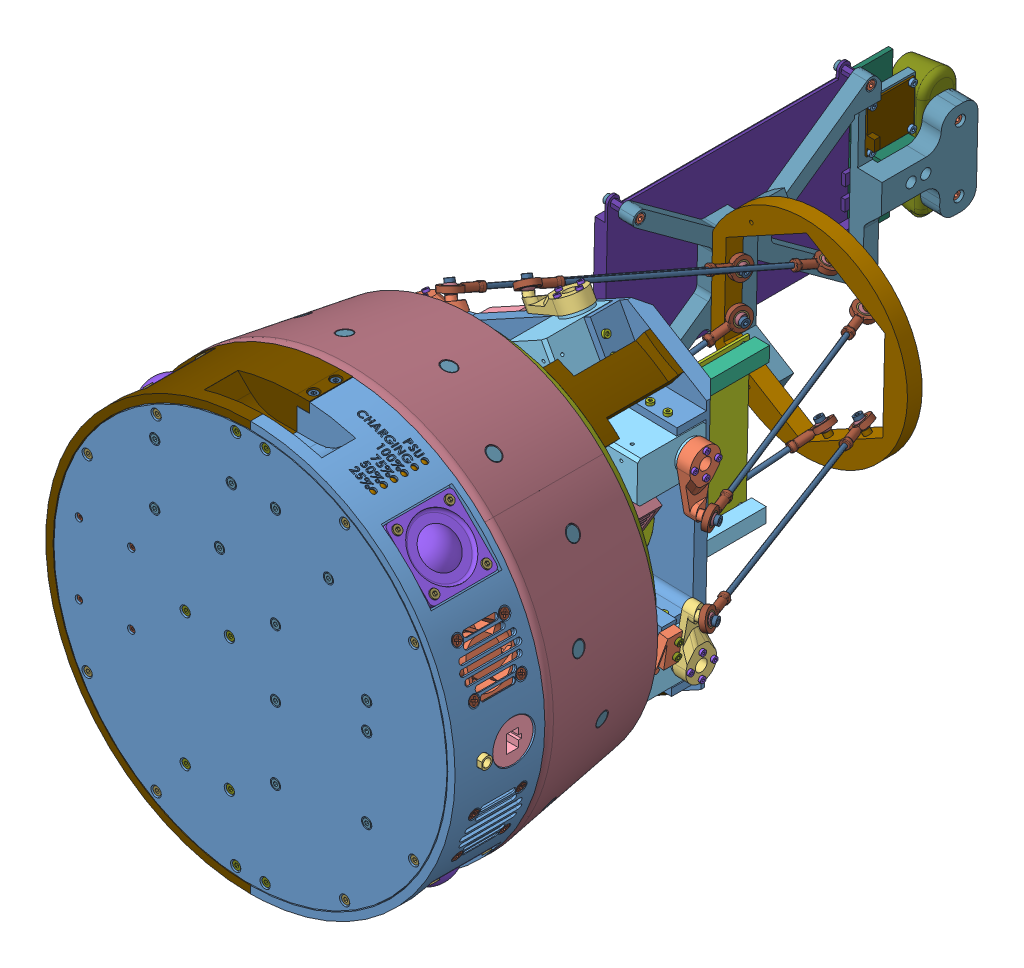
SolidWorks assembly robot, configuration Défaut. Lengths in mm. (continued)
Components (placement in the parent): (continued)
- stewart-1: stewart [Défaut] at (-73.8927 -28.7791 -12.2571) x (-0.023118 -0.999733 0) z (0 0 1) size (242.48 224.83 213.52)
  - stewart bottom-1: stewart bottom [Défaut] at (6.7039 12.5905 32.3281) size (242.48 216.75 132.5)
    - stewart bottom-1: stewart bottom [Défaut] at (-52.7025 18.5554 219.9038) size (234.9 203.43 30)
    - XL430-W250-T-1: XL430-W250-T [Défaut] at (-127.7192 44.5266 253.1538) x (-0.5 0.866025 0) z (-0.866025 -0.5 0) size (28.5 46.5 36)
    - XL430-W250-T-2: XL430-W250-T [Défaut] at (-112.7025 70.5362 253.1538) x (1 0 0) z (0 1 0) size (28.5 46.5 36)
    - XL430-W250-T-3: XL430-W250-T [Défaut] at (7.2975 70.5362 253.1538) x (1 0 0) z (0 1 0) size (28.5 46.5 36)
    - XL430-W250-T-4: XL430-W250-T [Défaut] at (22.3142 44.5266 253.1538) x (-0.5 -0.866025 0) z (0.866025 -0.5 0) size (28.5 46.5 36)
    - XL430-W250-T-5: XL430-W250-T [Défaut] at (-37.6858 -59.3965 253.1538) x (-0.5 -0.866025 0) z (0.866025 -0.5 0) size (28.5 46.5 36)
    - XL430-W250-T-6: XL430-W250-T [Défaut] at (-67.7192 -59.3965 253.1538) x (-0.5 0.866025 0) z (-0.866025 -0.5 0) size (28.5 46.5 36)
    - stewart horn (left)-1: stewart horn (left) [Défaut] at (-112.7025 116.5362 241.1538) x (1 0 0) z (0 -1 0) size (45.5 21 11.31)
    - stewart horn (right)-1: stewart horn (right) [Défaut] at (7.2975 116.5362 241.1538) x (-1 0 0) z (0 -1 0) size (45.5 21 11.31)
    - USB hub support-1: USB hub support [Défaut] at (-103.8877 -42.7506 219.9038) x (-0.866025 -0.5 0) z (0.5 -0.866025 0) size (24.57 17.21 30)
    - USB hub support-2: USB hub support [Défaut] at (-136.8877 14.407 219.9038) x (-0.866025 -0.5 0) z (0.5 -0.866025 0) size (24.57 17.21 30)
    - USB hub support-3: USB hub support [Défaut] at (-16.5172 -68.7314 219.9038) x (0.866025 -0.5 0) z (0.5 0.866025 0) size (24.57 17.21 30)
    - USB hub support-4: USB hub support [Défaut] at (16.4828 -11.5737 219.9038) x (0.866025 -0.5 0) z (0.5 0.866025 0) size (24.57 17.21 30)
    - OpenCR support 1-1: OpenCR support 1 [Défaut] at (-9.7025 62.0362 219.9038) x (-1 0 0) z (0 -1 0) size (20 76 23)
    - OpenCR support 2-1: OpenCR support 2 [Défaut] at (-95.7025 62.0362 219.9038) x (-1 0 0) z (0 -1 0) size (20 76 23)
    - OpenCR-1: OpenCR [Défaut] at (-52.7025 47.4362 181.9038) x (1 0 0) z (0 1 0) size (110.25 75 17.6)
    - Anker USB-c hub (4 ports)-1: Anker USB-c hub (4 ports) [Défaut] at (3.7083 -8.7432 211.4339) x (-0.5 -0.866025 0) z (-0.496732 0.286788 -0.819152) size (96 30 21)
    - Anker USB-c hub (4 ports)-2: Anker USB-c hub (4 ports) [Défaut] at (-109.4441 -8.9342 211.1664) x (0.5 -0.866025 0) z (0.496732 0.286788 -0.819152) size (96 30 21)
    - M2.5x8mm plastic-1: M2.5x8mm plastic [Défaut] at (-0.7025 93.5362 232.1538) x (-1 0 0) z (0 0 -1) size (4.5 4.5 9.9)
    - M2.5x8mm plastic-2: M2.5x8mm plastic [Défaut] at (15.2975 93.5362 232.1538) x (-1 0 0) z (0 0 -1) size (4.5 4.5 9.9)
    - M2.5x8mm plastic-3: M2.5x8mm plastic [Défaut] at (46.2328 39.9548 232.1538) x (-1 0 0) z (0 0 -1) size (4.5 4.5 9.9)
    - M2.5x8mm plastic-4: M2.5x8mm plastic [Défaut] at (38.2328 26.0984 232.1538) x (-1 0 0) z (0 0 -1) size (4.5 4.5 9.9)
    - M2.5x8mm plastic-5: M2.5x8mm plastic [Défaut] at (19.2975 93.5362 245.1538) x (0 -0.924225 -0.381849) z (1 0 0) size (4.5 4.5 9.9)
    - M2.5x8mm plastic-6: M2.5x8mm plastic [Défaut] at (19.2975 81.5362 245.1538) x (0 0 1) z (1 0 0) size (4.5 4.5 9.9)
    - M2.5x8mm plastic-7: M2.5x8mm plastic [Défaut] at (37.8404 49.4189 245.1538) x (0.75 -0.433013 -0.5) z (0.5 0.866025 0) size (4.5 4.5 9.9)
    - M2.5x8mm plastic-8: M2.5x8mm plastic [Défaut] at (48.2328 43.4189 245.1538) x (0.75 -0.433013 -0.5) z (0.5 0.866025 0) size (4.5 4.5 9.9)
    - M2.5x8mm plastic-9: M2.5x8mm plastic [Défaut] at (-4.7025 93.5362 245.1538) x (0 0 1) z (-1 0 0) size (4.5 4.5 9.9)
    - M2.5x8mm plastic-10: M2.5x8mm plastic [Défaut] at (-4.7025 81.5362 245.1538) x (0 0 1) z (-1 0 0) size (4.5 4.5 9.9)
    - M2.5x8mm plastic-11: M2.5x8mm plastic [Défaut] at (36.2328 22.6343 245.1538) x (-0.75 0.433013 -0.5) z (-0.5 -0.866025 0) size (4.5 4.5 9.9)
    - M2.5x8mm plastic-12: M2.5x8mm plastic [Défaut] at (25.8404 28.6343 245.1538) x (-0.75 0.433013 -0.5) z (-0.5 -0.866025 0) size (4.5 4.5 9.9)
    - M2x12mm socket-1: M2x12mm socket [Défaut] at (-112.7025 103.5362 233.1538) x (1 0 0) z (0 1 0) size (3.8 3.8 13.6)
    - M2x12mm socket-2: M2x12mm socket [Défaut] at (-104.7025 103.5362 241.1538) x (1 0 0) z (0 1 0) size (3.8 3.8 13.6)
    - M2x12mm socket-3: M2x12mm socket [Défaut] at (-112.7025 103.5362 249.1538) x (1 0 0) z (0 1 0) size (3.8 3.8 13.6)
    - M2x12mm socket-4: M2x12mm socket [Défaut] at (-120.7025 103.5362 241.1538) x (1 0 0) z (0 1 0) size (3.8 3.8 13.6)
    - M2x12mm socket-5: M2x12mm socket [Défaut] at (7.2975 103.5362 233.1538) x (1 0 0) z (0 1 0) size (3.8 3.8 13.6)
    - M2x12mm socket-6: M2x12mm socket [Défaut] at (-0.7025 103.5362 241.1538) x (1 0 0) z (0 1 0) size (3.8 3.8 13.6)
    - M2x12mm socket-7: M2x12mm socket [Défaut] at (7.2975 103.5362 249.1538) x (1 0 0) z (0 1 0) size (3.8 3.8 13.6)
    - M2x12mm socket-8: M2x12mm socket [Défaut] at (15.2975 103.5362 241.1538) x (1 0 0) z (0 1 0) size (3.8 3.8 13.6)
    - M3x12mm plastic-1: M3x12mm plastic [Défaut] at (-126.6425 11.6619 225.9038) x (-0.923728 -0.383049 0) z (0 0 -1) size (5.5 5.5 14.3)
    - M3x12mm plastic-2: M3x12mm plastic [Défaut] at (-119.1425 -1.3285 225.9038) x (-0.923728 -0.383049 0) z (0 0 -1) size (5.5 5.5 14.3)
    - M3x12mm plastic-3: M3x12mm plastic [Défaut] at (-93.6425 -45.4958 225.9038) x (-1 0 0) z (0 0 -1) size (5.5 5.5 14.3)
    - M3x12mm plastic-4: M3x12mm plastic [Défaut] at (-86.1425 -58.4862 225.9038) x (-1 0 0) z (0 0 -1) size (5.5 5.5 14.3)
    - M3x12mm plastic-5: M3x12mm plastic [Défaut] at (-19.2624 -58.4862 225.9038) x (-1 0 0) z (0 0 -1) size (5.5 5.5 14.3)
    - M3x12mm plastic-6: M3x12mm plastic [Défaut] at (-11.7624 -45.4958 225.9038) x (-0.923728 -0.383049 0) z (0 0 -1) size (5.5 5.5 14.3)
    - M3x12mm plastic-7: M3x12mm plastic [Défaut] at (13.7376 -1.3285 225.9038) x (-1 0 0) z (0 0 -1) size (5.5 5.5 14.3)
    - M3x12mm plastic-8: M3x12mm plastic [Défaut] at (21.2376 11.6619 225.9038) x (-1 0 0) z (0 0 -1) size (5.5 5.5 14.3)
    - M3x12mm plastic-9: M3x12mm plastic [Défaut] at (-110.7025 57.0362 225.9038) x (-0.923728 -0.383049 0) z (0 0 -1) size (5.5 5.5 14.3)
    - M3x12mm plastic-10: M3x12mm plastic [Défaut] at (-100.7025 67.0362 225.9038) x (-1 0 0) z (0 0 -1) size (5.5 5.5 14.3)
    - M3x12mm plastic-11: M3x12mm plastic [Défaut] at (-4.7025 67.0362 225.9038) x (-1 0 0) z (0 0 -1) size (5.5 5.5 14.3)
    - M3x12mm plastic-12: M3x12mm plastic [Défaut] at (5.2975 57.0362 225.9038) x (-1 0 0) z (0 0 -1) size (5.5 5.5 14.3)
    - M3x8mm plastic-1: M3x8mm plastic [Défaut] at (-4.7025 55.4362 148.9038) x (1 0 0) z (0 -1 0) size (5.5 5.5 10.3)
    - M3x8mm plastic-2: M3x8mm plastic [Défaut] at (-100.7025 55.4362 148.9038) x (1 0 0) z (0 -1 0) size (5.5 5.5 10.3)
    - M3x8mm plastic-3: M3x8mm plastic [Défaut] at (-100.7025 55.4362 214.9038) x (1 0 0) z (0 -1 0) size (5.5 5.5 10.3)
    - M3x8mm plastic-4: M3x8mm plastic [Défaut] at (-4.7025 55.4362 214.9038) x (1 0 0) z (0 -1 0) size (5.5 5.5 10.3)
    - M2.5x8mm plastic-13: M2.5x8mm plastic [Défaut] at (-21.7672 -77.8247 232.1538) x (0.5 0.866025 0) z (0 0 -1) size (4.5 4.5 9.9)
    - M2.5x8mm plastic-14: M2.5x8mm plastic [Défaut] at (-151.6377 39.9548 232.1538) x (0.5 -0.866025 0) z (0 0 -1) size (4.5 4.5 9.9)
    - M2.5x8mm plastic-15: M2.5x8mm plastic [Défaut] at (-83.6377 -77.8247 232.1538) x (0.5 0.866025 0) z (0 0 -1) size (4.5 4.5 9.9)
    - M2.5x8mm plastic-16: M2.5x8mm plastic [Défaut] at (-120.7025 93.5362 232.1538) x (0.5 -0.866025 0) z (0 0 -1) size (4.5 4.5 9.9)
    - M2.5x8mm plastic-17: M2.5x8mm plastic [Défaut] at (-91.6377 -63.9683 232.1538) x (0.5 0.866025 0) z (0 0 -1) size (4.5 4.5 9.9)
    - M2.5x8mm plastic-18: M2.5x8mm plastic [Défaut] at (-104.7025 93.5362 232.1538) x (0.5 -0.866025 0) z (0 0 -1) size (4.5 4.5 9.9)
    - M2.5x8mm plastic-19: M2.5x8mm plastic [Défaut] at (-23.7672 -81.2888 245.1538) x (-0.800402 0.462112 -0.381849) z (-0.5 -0.866025 0) size (4.5 4.5 9.9)
    - M2.5x8mm plastic-20: M2.5x8mm plastic [Défaut] at (-153.6377 43.4189 245.1538) x (0.800402 0.462112 -0.381849) z (-0.5 0.866025 0) size (4.5 4.5 9.9)
    - M2.5x8mm plastic-21: M2.5x8mm plastic [Défaut] at (-34.1596 -75.2888 245.1538) x (0 0 1) z (-0.5 -0.866025 0) size (4.5 4.5 9.9)
    - M2.5x8mm plastic-22: M2.5x8mm plastic [Défaut] at (-143.2454 49.4189 245.1538) x (0 0 1) z (-0.5 0.866025 0) size (4.5 4.5 9.9)
    - M2.5x8mm plastic-23: M2.5x8mm plastic [Défaut] at (-71.2454 -75.2888 245.1538) x (-0.75 -0.433013 -0.5) z (0.5 -0.866025 0) size (4.5 4.5 9.9)
    - M2.5x8mm plastic-24: M2.5x8mm plastic [Défaut] at (-124.7025 81.5362 245.1538) x (0 0.866025 -0.5) z (-1 0 0) size (4.5 4.5 9.9)
    - M2.5x8mm plastic-25: M2.5x8mm plastic [Défaut] at (-81.6377 -81.2888 245.1538) x (-0.75 -0.433013 -0.5) z (0.5 -0.866025 0) size (4.5 4.5 9.9)
    - M2.5x8mm plastic-26: M2.5x8mm plastic [Défaut] at (-124.7025 93.5362 245.1538) x (0 0.866025 -0.5) z (-1 0 0) size (4.5 4.5 9.9)
    - M2.5x8mm plastic-27: M2.5x8mm plastic [Défaut] at (-11.7672 -60.5042 245.1538) x (0 0 1) z (0.5 0.866025 0) size (4.5 4.5 9.9)
    - M2.5x8mm plastic-28: M2.5x8mm plastic [Défaut] at (-141.6377 22.6343 245.1538) x (0 0 1) z (0.5 -0.866025 0) size (4.5 4.5 9.9)
    - M2.5x8mm plastic-29: M2.5x8mm plastic [Défaut] at (-22.1596 -54.5042 245.1538) x (0 0 1) z (0.5 0.866025 0) size (4.5 4.5 9.9)
    - M2.5x8mm plastic-30: M2.5x8mm plastic [Défaut] at (-131.2454 28.6343 245.1538) x (0 0 1) z (0.5 -0.866025 0) size (4.5 4.5 9.9)
    - M2.5x8mm plastic-31: M2.5x8mm plastic [Défaut] at (-93.6377 -60.5042 245.1538) x (0.75 0.433013 -0.5) z (-0.5 0.866025 0) size (4.5 4.5 9.9)
    - M2.5x8mm plastic-32: M2.5x8mm plastic [Défaut] at (-100.7025 93.5362 245.1538) x (0 -0.866025 -0.5) z (1 0 0) size (4.5 4.5 9.9)
    - M2.5x8mm plastic-33: M2.5x8mm plastic [Défaut] at (-83.2454 -54.5042 245.1538) x (0.75 0.433013 -0.5) z (-0.5 0.866025 0) size (4.5 4.5 9.9)
    - M2.5x8mm plastic-34: M2.5x8mm plastic [Défaut] at (-100.7025 81.5362 245.1538) x (0 -0.866025 -0.5) z (1 0 0) size (4.5 4.5 9.9)
    - M2.5x8mm plastic-35: M2.5x8mm plastic [Défaut] at (-13.7672 -63.9683 232.1538) x (0.5 0.866025 0) z (0 0 -1) size (4.5 4.5 9.9)
    - M2.5x8mm plastic-36: M2.5x8mm plastic [Défaut] at (-143.6377 26.0984 232.1538) x (0.5 -0.866025 0) z (0 0 -1) size (4.5 4.5 9.9)
    - M2x12mm socket-9: M2x12mm socket [Défaut] at (-9.107 -75.8965 249.1538) x (-0.5 -0.866025 0) z (0.866025 -0.5 0) size (3.8 3.8 13.6)
    - M2x12mm socket-10: M2x12mm socket [Défaut] at (-156.298 28.0266 249.1538) x (-0.5 0.866025 0) z (-0.866025 -0.5 0) size (3.8 3.8 13.6)
    - M2x12mm socket-11: M2x12mm socket [Défaut] at (-13.107 -82.8247 241.1538) x (-0.5 -0.866025 0) z (0.866025 -0.5 0) size (3.8 3.8 13.6)
    - M2x12mm socket-12: M2x12mm socket [Défaut] at (-160.298 34.9548 241.1538) x (-0.5 0.866025 0) z (-0.866025 -0.5 0) size (3.8 3.8 13.6)
    - M2x12mm socket-13: M2x12mm socket [Défaut] at (-9.107 -75.8965 233.1538) x (-0.5 -0.866025 0) z (0.866025 -0.5 0) size (3.8 3.8 13.6)
    - M2x12mm socket-14: M2x12mm socket [Défaut] at (-156.298 28.0266 233.1538) x (-0.5 0.866025 0) z (-0.866025 -0.5 0) size (3.8 3.8 13.6)
    - M2x12mm socket-15: M2x12mm socket [Défaut] at (-5.107 -68.9683 241.1538) x (-0.5 -0.866025 0) z (0.866025 -0.5 0) size (3.8 3.8 13.6)
    - M2x12mm socket-16: M2x12mm socket [Défaut] at (-152.298 21.0984 241.1538) x (-0.5 0.866025 0) z (-0.866025 -0.5 0) size (3.8 3.8 13.6)
    - stewart horn (right)-2: stewart horn (right) [Défaut] at (2.1513 -82.3965 241.1538) x (0.5 0.866025 0) z (-0.866025 0.5 0) size (45.5 21 11.31)
    - stewart horn (right)-3: stewart horn (right) [Défaut] at (-167.5563 21.5266 241.1538) x (0.5 -0.866025 0) z (0.866025 0.5 0) size (45.5 21 11.31)
    - M2x12mm socket-17: M2x12mm socket [Défaut] at (54.893 34.9548 241.1538) x (-0.5 -0.866025 0) z (0.866025 -0.5 0) size (3.8 3.8 13.6)
    - M2x12mm socket-18: M2x12mm socket [Défaut] at (-92.298 -82.8247 241.1538) x (-0.5 0.866025 0) z (-0.866025 -0.5 0) size (3.8 3.8 13.6)
    - M2x12mm socket-19: M2x12mm socket [Défaut] at (50.893 28.0266 249.1538) x (-0.5 -0.866025 0) z (0.866025 -0.5 0) size (3.8 3.8 13.6)
    - M2x12mm socket-20: M2x12mm socket [Défaut] at (-96.298 -75.8965 249.1538) x (-0.5 0.866025 0) z (-0.866025 -0.5 0) size (3.8 3.8 13.6)
    - M2x12mm socket-21: M2x12mm socket [Défaut] at (46.893 21.0984 241.1538) x (-0.5 -0.866025 0) z (0.866025 -0.5 0) size (3.8 3.8 13.6)
    - M2x12mm socket-22: M2x12mm socket [Défaut] at (-100.298 -68.9683 241.1538) x (-0.5 0.866025 0) z (-0.866025 -0.5 0) size (3.8 3.8 13.6)
    - M2x12mm socket-23: M2x12mm socket [Défaut] at (50.893 28.0266 233.1538) x (-0.5 -0.866025 0) z (0.866025 -0.5 0) size (3.8 3.8 13.6)
    - M2x12mm socket-24: M2x12mm socket [Défaut] at (-96.298 -75.8965 233.1538) x (-0.5 0.866025 0) z (-0.866025 -0.5 0) size (3.8 3.8 13.6)
    - stewart horn (left)-4: stewart horn (left) [Défaut] at (62.1513 21.5266 241.1538) x (-0.5 -0.866025 0) z (-0.866025 0.5 0) size (45.5 21 11.31)
    - stewart horn (left)-5: stewart horn (left) [Défaut] at (-107.5563 -82.3965 241.1538) x (-0.5 0.866025 0) z (0.866025 0.5 0) size (45.5 21 11.31)
  - stewart top-1: stewart top [Défaut] at (-45.9986 31.146 97.8209) x (-1 0 0) z (0 0 1) size (140 133 10)
  - stewart rod-1: stewart rod [Défaut] at (-79.2175 71.5134 114.2702) x (0.856661 -0.487567 0.168555) z (0.018875 0.356138 0.934243) size (3 3 160)
  - stewart rod-2: stewart rod [Défaut] at (-97.5673 39.7307 114.2702) x (0.953731 -0.028379 0.299318) z (-0.298987 -0.194416 0.934243) size (3 3 160)
  - ball joint-1: ball joint [Défaut] at (-80.6822 62.9327 84.0597) x (0.317889 0.883784 -0.343326) z (0.018875 0.356138 0.934243) size (14 8.06 27.54) (flexible)
    - ball joint body-1: ball joint body [Défaut] at (-2.323 -1.7007 27.3075) size (14 5.52 27.54)
    - ball joint liner-1: ball joint liner [Défaut] at (-2.323 -1.7007 20.7692) size (9 3.5 9)
    - ball joint ball-1: ball joint ball [Défaut] at (-2.323 -1.7007 20.7692) x (-0.700869 0.159426 -0.695245) z (0.677471 -0.156207 -0.718771) size (8 6 8)
  - ball joint-2: ball joint [Défaut] at (-89.2244 48.5004 85.254) x (0.238407 0.932761 0.270405) z (-0.298987 -0.194416 0.934243) size (14 8.06 27.54) (flexible)
    - ball joint body-1: ball joint body [Défaut] at (-2.323 -1.7007 27.3075) size (14 5.52 27.54)
    - ball joint liner-1: ball joint liner [Défaut] at (-2.323 -1.7007 20.7692) x (0.902027 0 -0.43168) z (0.43168 0 0.902027) size (9 3.5 9)
    - ball joint ball-1: ball joint ball [Défaut] at (-2.323 -1.7007 20.7692) x (-0.869039 0.186885 0.458088) z (-0.448198 0.094688 -0.888905) size (8 6 8)
  - ball joint-3: ball joint [Défaut] at (-155.0744 5.358 293.486) x (-0.64664 0.76125 -0.048529) z (0.298987 0.194416 -0.934243) size (14 8.06 27.54) (flexible)
    - ball joint body-1: ball joint body [Défaut] at (-2.323 -1.7007 27.3075) size (14 5.52 27.54)
    - ball joint liner-1: ball joint liner [Défaut] at (-2.323 -1.7007 20.7692) x (-0.995574 0 0.093986) z (-0.093986 0 -0.995574) size (9 3.5 9)
    - ball joint ball-1: ball joint ball [Défaut] at (-2.323 -1.7007 20.7692) x (0.752494 0.12262 0.647084) z (-0.631975 -0.142099 0.76185) size (8 6 8)
  - ball joint-4: ball joint [Défaut] at (-77.7502 141.4551 292.3512) x (-0.994952 0.098799 -0.017561) z (-0.018875 -0.356138 -0.934243) size (14 8.06 27.54) (flexible)
    - ball joint body-1: ball joint body [Défaut] at (-2.323 -1.7007 27.3075) size (14 5.52 27.54)
    - ball joint liner-1: ball joint liner [Défaut] at (-2.323 -1.7007 20.7692) x (-0.999882 0 0.015364) z (-0.015364 0 -0.999882) size (9 3.5 9)
    - ball joint ball-1: ball joint ball [Défaut] at (-2.323 -1.7007 20.7692) x (0.696255 -0.090433 -0.712075) z (0.710923 -0.05006 0.701486) size (8 6 8)
  - stewart rod-3: stewart rod [Défaut] at (-12.7796 71.5134 114.2702) x (-0.501443 -0.811766 0.299318) z (-0.018875 0.356138 0.934243) size (3 3 160)
  - stewart rod-4: stewart rod [Défaut] at (-27.6489 -17.8062 114.2702) x (-0.452288 0.840145 0.299318) z (0.317862 -0.161723 0.934243) size (3 3 160)
  - ball joint-5: ball joint [Défaut] at (-1.1286 45.2895 84.0597) x (0.606435 -0.717192 -0.343326) z (0.298987 -0.194416 0.934243) size (14 8.06 27.54) (flexible)
    - ball joint body-1: ball joint body [Défaut] at (-2.323 -1.7007 27.3075) size (14 5.52 27.54)
    - ball joint liner-1: ball joint liner [Défaut] at (-2.323 -1.7007 20.7692) x (0.973602 0 0.228251) z (-0.228251 0 0.973602) size (9 3.5 9)
    - ball joint ball-1: ball joint ball [Défaut] at (-2.323 -1.7007 20.7692) x (-0.483951 0.20175 -0.851521) z (0.869766 0.003667 -0.493451) size (8 6 8)
  - ball joint-6: ball joint [Défaut] at (-56.1849 -14.7843 84.0597) x (-0.924324 -0.166592 -0.343326) z (-0.317862 -0.161723 0.934243) size (14 8.06 27.54) (flexible)
    - ball joint body-1: ball joint body [Défaut] at (-2.323 -1.7007 27.3075) size (14 5.52 27.54)
    - ball joint liner-1: ball joint liner [Défaut] at (-2.323 -1.7007 20.7692) x (0.976476 0 0.215624) z (-0.215624 0 0.976476) size (9 3.5 9)
    - ball joint ball-1: ball joint ball [Défaut] at (-2.323 -1.7007 20.7692) x (-0.494633 0.20169 -0.845375) z (0.863736 0.006153 -0.503908) size (8 6 8)
  - ball joint-7: ball joint [Défaut] at (-9.3563 59.9034 85.254) x (0.688591 -0.672847 0.270405) z (-0.018875 0.356138 0.934243) size (14 8.06 27.54) (flexible)
    - ball joint body-1: ball joint body [Défaut] at (-2.323 -1.7007 27.3075) size (14 5.52 27.54)
    - ball joint liner-1: ball joint liner [Défaut] at (-2.323 -1.7007 20.7692) x (0.902027 0 -0.43168) z (0.43168 0 0.902027) size (9 3.5 9)
    - ball joint ball-1: ball joint ball [Défaut] at (-2.323 -1.7007 20.7692) x (-0.826872 0.184645 -0.531214) z (0.553406 0.098985 -0.827009) size (8 6 8)
  - ball joint-8: ball joint [Défaut] at (-39.4151 -14.9659 85.254) x (-0.926998 -0.259914 0.270405) z (0.317862 -0.161723 0.934243) size (14 8.06 27.54) (flexible)
    - ball joint body-1: ball joint body [Défaut] at (-2.323 -1.7007 27.3075) size (14 5.52 27.54)
    - ball joint liner-1: ball joint liner [Défaut] at (-2.323 -1.7007 20.7692) x (0.902027 0 -0.43168) z (0.43168 0 0.902027) size (9 3.5 9)
    - ball joint ball-1: ball joint ball [Défaut] at (-2.323 -1.7007 20.7692) x (-0.826872 0.184645 -0.531214) z (0.553406 0.098985 -0.827009) size (8 6 8)
  - ball joint-9: ball joint [Défaut] at (-13.7937 138.5023 293.486) x (0.982582 0.179382 -0.048529) z (0.018875 -0.356138 -0.934243) size (14 8.06 27.54) (flexible)
    - ball joint body-1: ball joint body [Défaut] at (-2.323 -1.7007 27.3075) size (14 5.52 27.54)
    - ball joint liner-1: ball joint liner [Défaut] at (-2.323 -1.7007 20.7692) x (-0.988912 0 0.148502) z (-0.148502 0 -0.988912) size (9 3.5 9)
    - ball joint ball-1: ball joint ball [Défaut] at (-2.323 -1.7007 20.7692) x (0.807961 -0.168555 0.564613) z (-0.582369 -0.082565 0.808721) size (8 6 8)
  - ball joint-10: ball joint [Défaut] at (30.8723 -50.4225 293.486) x (-0.335942 -0.940632 -0.048529) z (-0.317862 0.161723 -0.934243) size (14 8.06 27.54) (flexible)
    - ball joint body-1: ball joint body [Défaut] at (-2.323 -1.7007 27.3075) size (14 5.52 27.54)
    - ball joint liner-1: ball joint liner [Défaut] at (-2.323 -1.7007 20.7692) x (-0.999973 0 0.007391) z (-0.007391 0 -0.999973) size (9 3.5 9)
    - ball joint ball-1: ball joint ball [Défaut] at (-2.323 -1.7007 20.7692) x (0.711735 -0.179011 0.679256) z (-0.696698 -0.056417 0.715143) size (8 6 8)
  - ball joint-11: ball joint [Défaut] at (65.4077 3.4891 292.3512) x (0.583038 0.812255 -0.017561) z (-0.298987 0.194416 -0.934243) size (14 8.06 27.54) (flexible)
    - ball joint body-1: ball joint body [Défaut] at (-2.323 -1.7007 27.3075) size (14 5.52 27.54)
    - ball joint liner-1: ball joint liner [Défaut] at (-2.323 -1.7007 20.7692) x (-0.999862 0 -0.016633) z (0.016633 0 -0.999862) size (9 3.5 9)
    - ball joint ball-1: ball joint ball [Défaut] at (-2.323 -1.7007 20.7692) x (0.67574 -0.100225 0.730295) z (-0.735483 -0.02528 0.677071) size (8 6 8)
  - ball joint-12: ball joint [Défaut] at (-125.6533 -51.5063 292.3512) x (0.411914 -0.911053 -0.017561) z (0.317862 0.161723 -0.934243) size (14 8.06 27.54) (flexible)
    - ball joint body-1: ball joint body [Défaut] at (-2.323 -1.7007 27.3075) size (14 5.52 27.54)
    - ball joint liner-1: ball joint liner [Défaut] at (-2.323 -1.7007 20.7692) x (-0.999451 0 0.033133) z (-0.033133 0 -0.999451) size (9 3.5 9)
    - ball joint ball-1: ball joint ball [Défaut] at (-2.323 -1.7007 20.7692) x (0.709778 -0.098917 0.697446) z (-0.702692 -0.029993 0.710862) size (8 6 8)
  - stewart rod-5: stewart rod [Défaut] at (5.5701 39.7307 114.2702) x (-0.850576 -0.498107 0.168555) z (0.298987 -0.194416 0.934243) size (3 3 160)
  - stewart rod-6: stewart rod [Défaut] at (-64.3483 -17.8062 114.2702) x (-0.006085 0.985673 0.168555) z (-0.317862 -0.161723 0.934243) size (3 3 160)
  - M3x12mm plastic-1: M3x12mm plastic [Défaut] at (-141.1945 10.8256 276.5512) x (0.003597 -0.575273 0.817953) z (-0.817953 -0.472246 -0.328537) size (5.5 5.5 14.3)
  - M3x12mm plastic-2: M3x12mm plastic [Défaut] at (-75.9986 123.7482 276.5512) x (0.011237 0.328516 0.944431) z (0 0.944491 -0.328537) size (5.5 5.5 14.3)
  - M3x12mm plastic-3: M3x12mm plastic [Défaut] at (-102.0944 46.2124 102.8759) x (-0.115621 -0.500129 -0.858198) z (0.853104 -0.49254 0.172101) size (5.5 5.5 14.3)
  - M3x12mm plastic-4: M3x12mm plastic [Défaut] at (-87.0944 72.1931 102.8759) x (0.508145 0.709554 -0.488183) z (0.853104 -0.49254 0.172101) size (5.5 5.5 14.3)
  - M3x12mm plastic-5: M3x12mm plastic [Défaut] at (10.0972 46.2124 102.8759) x (0.360419 -0.794843 -0.488183) z (-0.853104 -0.49254 0.172101) size (5.5 5.5 14.3)
  - M3x12mm plastic-6: M3x12mm plastic [Défaut] at (-60.9986 -24.9676 102.8759) x (-0.868564 0.085289 -0.488183) z (0 0.985079 0.172101) size (5.5 5.5 14.3)
  - M3x12mm plastic-7: M3x12mm plastic [Défaut] at (-4.9028 72.1931 102.8759) x (-0.375314 0.350195 -0.858198) z (-0.853104 -0.49254 0.172101) size (5.5 5.5 14.3)
  - M3x12mm plastic-8: M3x12mm plastic [Défaut] at (-30.9986 -24.9676 102.8759) x (0.490935 0.149934 -0.858198) z (0 0.985079 0.172101) size (5.5 5.5 14.3)
  - M3x12mm plastic-9: M3x12mm plastic [Défaut] at (49.1973 10.8256 276.5512) x (0.278885 -0.17399 0.944431) z (0.817953 -0.472246 -0.328537) size (5.5 5.5 14.3)
  - M3x12mm plastic-10: M3x12mm plastic [Défaut] at (-111.1945 -41.1359 276.5512) x (-0.290122 -0.154526 0.944431) z (-0.817953 -0.472246 -0.328537) size (5.5 5.5 14.3)
  - M3x12mm plastic-11: M3x12mm plastic [Défaut] at (-15.9986 123.7482 276.5512) x (-0.5 0.284521 0.817953) z (0 0.944491 -0.328537) size (5.5 5.5 14.3)
  - M3x12mm plastic-12: M3x12mm plastic [Défaut] at (19.1973 -41.1359 276.5512) x (0.496403 0.290752 0.817953) z (0.817953 -0.472246 -0.328537) size (5.5 5.5 14.3)
- head-1: head [Défaut] at (-77.6466 -5.9099 260.0082) x (-0.023118 -0.999733 0) z (0 0 -1) size (128.33 66.3 224.36)
  - head-1: head [Défaut] at (-23.2223 -35.4275 174.4445) size (128.33 46.8 223.89)
  - head cable protector-1: head cable protector [Défaut] at (-23.4875 51.0725 292.5758) x (1 0 0) z (0 -1 0) size (100 33 25)
  - Intel RealSense D435i-1: Intel RealSense D435i [Défaut] at (-23.2223 33.5725 321.3334) x (1 0 0) z (0 -1 0) size (90.36 24.95 25.31)
  - screen-1: screen [Défaut] at (-28.4523 45.5725 192.8445) x (0 0 1) z (0 1 0) size (166.25 124 16.51)
  - wide angle camera-1: wide angle camera [Défaut] at (-56.3573 32.5725 289.1237) x (1 0 0) z (0 -1 0) size (32 32 30.75)
  - M2.5x5mm plastic-2: M2.5x5mm plastic [Défaut] at (-70.1476 36.3225 275.3334) x (-1 0 0) z (0 -1 0) size (4.5 4.5 6.9)
  - M2.5x5mm plastic-3: M2.5x5mm plastic [Défaut] at (-42.567 36.3225 302.914) x (1 0 0) z (0 -1 0) size (4.5 4.5 6.9)
  - M2.5x5mm plastic-4: M2.5x5mm plastic [Défaut] at (-70.1476 36.3225 302.914) x (1 0 0) z (0 -1 0) size (4.5 4.5 6.9)
  - M3x12mm plastic-1: M3x12mm plastic [Défaut] at (-25.7223 35.0725 298.3334) x (1 0 0) z (0 -1 0) size (5.5 5.5 14.3)
  - M3x12mm plastic-2: M3x12mm plastic [Défaut] at (-25.7223 35.0725 288.3334) x (1 0 0) z (0 -1 0) size (5.5 5.5 14.3)
  - M3x10mm socket-1: M3x10mm socket [Défaut] at (-45.7223 30.8225 321.3334) x (1 0 0) z (0 -1 0) size (5.5 5.5 13)
  - M3x10mm socket-2: M3x10mm socket [Défaut] at (-0.7223 30.8225 321.3334) x (1 0 0) z (0 -1 0) size (5.5 5.5 13)
  - M3x5mm socket-1: M3x5mm socket [Défaut] at (-85.9923 42.2925 271.3445) x (1 0 0) z (0 1 0) size (5.5 5.5 8)
  - M3x5mm socket-2: M3x5mm socket [Défaut] at (29.0877 42.2925 271.3445) x (1 0 0) z (0 1 0) size (5.5 5.5 8)
  - M3x5mm socket-3: M3x5mm socket [Défaut] at (-85.9923 42.2925 114.4445) x (1 0 0) z (0 1 0) size (5.5 5.5 8)
  - M3x5mm socket-4: M3x5mm socket [Défaut] at (29.0877 42.2925 114.4445) x (1 0 0) z (0 1 0) size (5.5 5.5 8)
  - M3x10mm socket-3: M3x10mm socket [Défaut] at (-85.9923 40.5725 271.3445) x (1 0 0) z (0 -1 0) size (5.5 5.5 13)
  - M3x10mm socket-4: M3x10mm socket [Défaut] at (-85.9923 40.5725 114.4445) x (1 0 0) z (0 -1 0) size (5.5 5.5 13)
  - M3x10mm socket-5: M3x10mm socket [Défaut] at (29.0877 40.5725 114.4445) x (1 0 0) z (0 -1 0) size (5.5 5.5 13)
  - M3x10mm socket-6: M3x10mm socket [Défaut] at (29.0877 40.5725 271.3445) x (1 0 0) z (0 -1 0) size (5.5 5.5 13)
  - M2.5x5mm plastic-1: M2.5x5mm plastic [Défaut] at (-42.567 36.3225 275.3334) x (-1 0 0) z (0 -1 0) size (4.5 4.5 6.9)
- M3x12mm plastic-1: M3x12mm plastic [Défaut] at (67.3312 61.6315 336.9748) x (-1 0 0) z (0 0 -1) size (5.5 5.5 14.3)
- M3x12mm plastic-16: M3x12mm plastic [Défaut] at (76.3083 16.4739 336.9748) x (-0.92388 0.382683 0) z (0 0 -1) size (5.5 5.5 14.3)
- M3x12mm plastic-15: M3x12mm plastic [Défaut] at (67.321 -28.6817 336.9748) x (-0.707107 0.707107 0) z (0 0 -1) size (5.5 5.5 14.3)
- M3x12mm plastic-14: M3x12mm plastic [Défaut] at (41.7375 -66.9608 336.9748) x (-0.382683 0.92388 0) z (0 0 -1) size (5.5 5.5 14.3)
- M3x12mm plastic-13: M3x12mm plastic [Défaut] at (3.4527 -92.5357 336.9748) x (0 1 0) z (0 0 -1) size (5.5 5.5 14.3)
- M3x12mm plastic-12: M3x12mm plastic [Défaut] at (-41.705 -101.5128 336.9748) x (0.382683 0.92388 0) z (0 0 -1) size (5.5 5.5 14.3)
- M3x12mm plastic-11: M3x12mm plastic [Défaut] at (-86.8606 -92.5255 336.9748) x (0.707107 0.707107 0) z (0 0 -1) size (5.5 5.5 14.3)
- M3x12mm plastic-10: M3x12mm plastic [Défaut] at (-125.1397 -66.9421 336.9748) x (0.92388 0.382683 0) z (0 0 -1) size (5.5 5.5 14.3)
- M3x12mm plastic-9: M3x12mm plastic [Défaut] at (-150.7145 -28.6572 336.9748) x (1 0 0) z (0 0 -1) size (5.5 5.5 14.3)
- M3x12mm plastic-8: M3x12mm plastic [Défaut] at (-159.6917 16.5004 336.9748) x (0.92388 -0.382683 0) z (0 0 -1) size (5.5 5.5 14.3)
- M3x12mm plastic-7: M3x12mm plastic [Défaut] at (-150.7044 61.6561 336.9748) x (0.707107 -0.707107 0) z (0 0 -1) size (5.5 5.5 14.3)
- M3x12mm plastic-6: M3x12mm plastic [Défaut] at (-125.1209 99.9351 336.9748) x (0.382683 -0.92388 0) z (0 0 -1) size (5.5 5.5 14.3)
- M3x12mm plastic-5: M3x12mm plastic [Défaut] at (-86.8361 125.51 336.9748) x (0 -1 0) z (0 0 -1) size (5.5 5.5 14.3)
- M3x12mm plastic-4: M3x12mm plastic [Défaut] at (-41.6784 134.4872 336.9748) x (-0.382683 -0.92388 0) z (0 0 -1) size (5.5 5.5 14.3)
- M3x12mm plastic-3: M3x12mm plastic [Défaut] at (3.4772 125.4999 336.9748) x (-0.707107 -0.707107 0) z (0 0 -1) size (5.5 5.5 14.3)
- M3x12mm plastic-2: M3x12mm plastic [Défaut] at (41.7563 99.9164 336.9748) x (-0.92388 -0.382683 0) z (0 0 -1) size (5.5 5.5 14.3)
- M3x12mm plastic-17: M3x12mm plastic [Défaut] at (-147.3369 11.4281 255.9748) x (-0.999997 0.002461 0) z (0 0 -1) size (5.5 5.5 14.3)
- M3x12mm plastic-18: M3x12mm plastic [Défaut] at (-146.9901 26.4241 255.9748) x (-0.999997 0.002461 0) z (0 0 -1) size (5.5 5.5 14.3)
- M3x12mm plastic-19: M3x12mm plastic [Défaut] at (2.3519 -79.6724 255.9748) x (-0.999997 0.002461 0) z (0 0 -1) size (5.5 5.5 14.3)
- M3x12mm plastic-20: M3x12mm plastic [Défaut] at (15.5122 -72.4747 255.9748) x (-0.999997 0.002461 0) z (0 0 -1) size (5.5 5.5 14.3)
- M3x12mm plastic-21: M3x12mm plastic [Défaut] at (6.7497 110.5081 255.9748) x (-0.999997 0.002461 0) z (0 0 -1) size (5.5 5.5 14.3)
- M3x12mm plastic-22: M3x12mm plastic [Défaut] at (19.5632 102.7098 255.9748) x (-0.999997 0.002461 0) z (0 0 -1) size (5.5 5.5 14.3)
- M3x12mm plastic-23: M3x12mm plastic [Défaut] at (-77.733 66.1596 91.5637) x (-0.986009 0.16669 0) z (0 0 -1) size (5.5 5.5 14.3)
- M3x12mm plastic-24: M3x12mm plastic [Défaut] at (-79.9905 -31.4662 91.5637) x (-0.98865 0.150239 0) z (0 0 -1) size (5.5 5.5 14.3)
- M3x12mm plastic-25: M3x12mm plastic [Défaut] at (-98.2141 37.7996 90.5637) x (-0.002718 -0.117533 0.993065) z (-0.999733 0.023118 0) size (5.5 5.5 14.3)
- M3x12mm plastic-26: M3x12mm plastic [Défaut] at (-99.1388 -2.1897 90.5637) x (-0.002718 -0.117533 0.993065) z (-0.999733 0.023118 0) size (5.5 5.5 14.3)
Mates (geometry in assembly coordinates):
- Coïncidente1: coincident anti-aligned: plane of base-1/base mic-1/base mic-1 through (-128.6528 103.4678 330.9748) normal (0 0 -1); plane of torso bottom-1/base gear-1 through (-41.6917 16.4872 330.9748) normal (0 0 1)
- Coaxiale1: concentric aligned: cylinder of base-1/base mic-1/base mic-2 through (76.3083 16.4739 337.9748) axis (0 0 -1) radius 1.25; cylinder of torso bottom-1/base gear-1 through (76.3083 16.4739 330.9758) axis (0 0 -1) radius 1.75
- Coaxiale2: concentric aligned: cylinder of base-1/base mic-1/base mic-2 through (67.321 -28.6817 337.9748) axis (0 0 -1) radius 1.25; cylinder of torso bottom-1/base gear-1 through (67.321 -28.6817 330.9758) axis (0 0 -1) radius 1.75
- Coaxiale3: concentric anti-aligned: cylinder of torso bottom-1/base gear-1 through (67.3312 61.6315 330.9758) axis (0 0 -1) radius 1.75; cylinder of M3x12mm plastic-1 through (67.3312 61.6315 324.9748) axis (0 0 1) radius 1.5
- Coïncidente2: coincident aligned: plane of torso bottom-1/base gear-1 through (67.3312 61.6315 324.9748) normal (0 0 -1); circle of M3x12mm plastic-1
- Coïncidente3: coincident anti-aligned: plane of torso bottom-1/stewart support-2 through (-41.6917 16.4872 249.9748) normal (0 0 -1); plane of stewart-1/stewart bottom-1/stewart bottom-1 through (-41.6917 16.4872 249.9748) normal (0 0 1)
- Coaxiale4: concentric aligned: cylinder of torso bottom-1/stewart support-2 through (-147.3369 11.4281 259.9748) axis (0 0 -1) radius 1.25; cylinder of stewart-1/stewart bottom-1/stewart bottom-1 through (-147.3369 11.4281 269.9758) axis (0 0 -1) radius 1.75
- Coaxiale5: concentric aligned: cylinder of torso bottom-1/stewart support-2 through (-146.9901 26.4241 259.9748) axis (0 0 -1) radius 1.25; cylinder of stewart-1/stewart bottom-1/stewart bottom-1 through (-146.9901 26.4241 269.9758) axis (0 0 -1) radius 1.75
- Coaxiale6: concentric anti-aligned: cylinder of stewart-1/stewart bottom-1/stewart bottom-1 through (-147.3369 11.4281 269.9758) axis (0 0 -1) radius 1.75; cylinder of M3x12mm plastic-17 through (-147.3369 11.4281 243.9748) axis (0 0 1) radius 1.5
- Coïncidente4: coincident aligned: plane of stewart-1/stewart bottom-1/stewart bottom-1 through (-147.3369 11.4281 243.9748) normal (0 0 -1); circle of M3x12mm plastic-17
- Coaxiale7: concentric anti-aligned: cylinder of stewart-1/stewart bottom-1/stewart bottom-1 through (-146.9901 26.4241 269.9758) axis (0 0 -1) radius 1.75; cylinder of M3x12mm plastic-18 through (-146.9901 26.4241 243.9748) axis (0 0 1) radius 1.5
- Coïncidente5: coincident aligned: plane of stewart-1/stewart bottom-1/stewart bottom-1 through (-146.9901 26.4241 243.9748) normal (0 0 -1); circle of M3x12mm plastic-18
- Coaxiale8: concentric anti-aligned: cylinder of stewart-1/stewart bottom-1/stewart bottom-1 through (2.3519 -79.6724 269.9758) axis (0 0 -1) radius 1.75; cylinder of M3x12mm plastic-19 through (2.3519 -79.6724 243.9748) axis (0 0 1) radius 1.5
- Coïncidente6: coincident aligned: plane of stewart-1/stewart bottom-1/stewart bottom-1 through (2.3519 -79.6724 243.9748) normal (0 0 -1); circle of M3x12mm plastic-19
- Coaxiale9: concentric anti-aligned: cylinder of stewart-1/stewart bottom-1/stewart bottom-1 through (15.5122 -72.4747 269.9758) axis (0 0 -1) radius 1.75; cylinder of M3x12mm plastic-20 through (15.5122 -72.4747 243.9748) axis (0 0 1) radius 1.5
- Coïncidente7: coincident aligned: plane of stewart-1/stewart bottom-1/stewart bottom-1 through (15.5122 -72.4747 243.9748) normal (0 0 -1); circle of M3x12mm plastic-20
- Coaxiale10: concentric anti-aligned: cylinder of stewart-1/stewart bottom-1/stewart bottom-1 through (6.7497 110.5081 269.9758) axis (0 0 -1) radius 1.75; cylinder of M3x12mm plastic-21 through (6.7497 110.5081 243.9748) axis (0 0 1) radius 1.5
- Coïncidente8: coincident aligned: plane of stewart-1/stewart bottom-1/stewart bottom-1 through (6.7497 110.5081 243.9748) normal (0 0 -1); circle of M3x12mm plastic-21
- Coaxiale11: concentric anti-aligned: cylinder of stewart-1/stewart bottom-1/stewart bottom-1 through (19.5632 102.7098 269.9758) axis (0 0 -1) radius 1.75; cylinder of M3x12mm plastic-22 through (19.5632 102.7098 243.9748) axis (0 0 1) radius 1.5
- Coïncidente9: coincident aligned: plane of stewart-1/stewart bottom-1/stewart bottom-1 through (19.5632 102.7098 243.9748) normal (0 0 -1); circle of M3x12mm plastic-22
- Coïncidente10: coincident anti-aligned: plane of head-1/head-1 through (-41.6917 16.4872 85.5637) normal (0 0 1); plane of stewart-1/stewart top-1 through (-41.6917 16.4872 85.5637) normal (0 0 -1)
- Coaxiale14: concentric aligned: cylinder of stewart-1/stewart top-1 through (-96.2146 37.7533 90.5637) axis (-0.999733 0.023118 0) radius 1.25; cylinder of head-1/head-1 through (-67.4206 37.0875 90.5637) axis (-0.999733 0.023118 0) radius 1.75
- Coaxiale15: concentric aligned: cylinder of stewart-1/stewart top-1 through (-97.1393 -2.236 90.5637) axis (-0.999733 0.023118 0) radius 1.25; cylinder of head-1/head-1 through (-68.3453 -2.9018 90.5637) axis (-0.999733 0.023118 0) radius 1.75
- Coïncidente11: coincident anti-aligned: plane of stewart-1/stewart top-1 through (-105.3802 -12.5605 95.5647) normal (-0.999733 0.023118 0); plane of head-1/head-1 through (-104.6748 17.9436 85.5637) normal (0.999733 -0.023118 0)
- Coaxiale16: concentric anti-aligned: cylinder of head-1/head-1 through (-79.9905 -31.4662 95.5647) axis (0 0 -1) radius 1.75; cylinder of M3x12mm plastic-24 through (-79.9905 -31.4662 79.5637) axis (0 0 1) radius 1.5
- Coïncidente12: coincident aligned: plane of head-1/head-1 through (-79.9905 -31.4662 79.5637) normal (0 0 -1); circle of M3x12mm plastic-24
- Coaxiale17: concentric anti-aligned: cylinder of head-1/head-1 through (-77.733 66.1596 95.5647) axis (0 0 -1) radius 1.75; cylinder of M3x12mm plastic-23 through (-77.733 66.1596 79.5637) axis (0 0 1) radius 1.5
- Coïncidente13: coincident aligned: plane of head-1/head-1 through (-77.733 66.1596 79.5637) normal (0 0 -1); circle of M3x12mm plastic-23
- Coaxiale18: concentric anti-aligned: cylinder of head-1/head-1 through (-68.3453 -2.9018 90.5637) axis (-0.999733 0.023118 0) radius 1.75; cylinder of M3x12mm plastic-26 through (-111.1356 -1.9123 90.5637) axis (0.999733 -0.023118 0) radius 1.5
- Coïncidente14: coincident aligned: plane of head-1/head-1 through (-111.1356 -1.9123 90.5637) normal (-0.999733 0.023118 0); circle of M3x12mm plastic-26
- Coaxiale19: concentric anti-aligned: cylinder of head-1/head-1 through (-67.4206 37.0875 90.5637) axis (-0.999733 0.023118 0) radius 1.75; cylinder of M3x12mm plastic-25 through (-110.2109 38.077 90.5637) axis (0.999733 -0.023118 0) radius 1.5
- Coïncidente15: coincident aligned: plane of head-1/head-1 through (-110.2109 38.077 90.5637) normal (-0.999733 0.023118 0); circle of M3x12mm plastic-25
